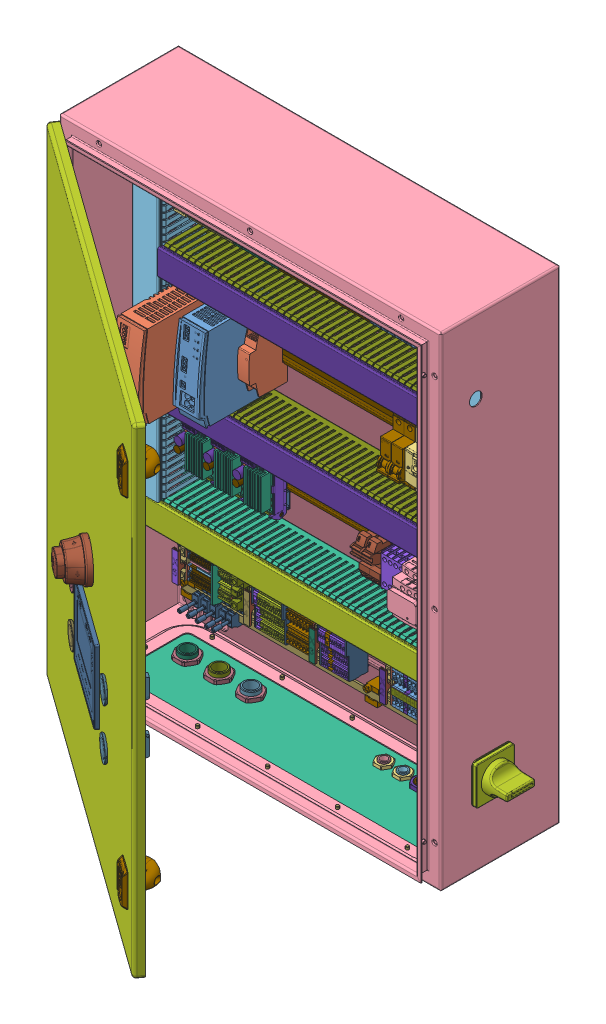
SolidWorks assembly Armoir életrique v46.step, configuration Valor predeterminado. Lengths in mm. (continued)
Components (placement in the parent): (continued)
- EM-241C_v4_1.step-1: EM-241C_v4_1.step [Valor predeterminado] at (-403.6882 -6.6708 82.3602) size (46 89.6 55.6) (continued)
  - DesignRootModel_1.step-1: DesignRootModel_1.step [Valor predeterminado] at origin size (42 72 25.9) (continued)
    - Submodel-RES0805_10K_part_simplified_0805_4.step-1: Submodel-RES0805_10K_part_simplified_0805_4.step [Valor predeterminado] at (555.4382 265.214 -26.9602) x (-1 0 0) z (0 0 1) size (2 1.25 0.6) (continued)
      - Submodel-C_UsersTino Hellbergworks3D kokeilujaEM-241Cver4_PCB3DInput_SRES 0805.xtd_76.step-1: Submodel-C_UsersTino Hellbergworks3D kokeilujaEM-241Cver4_PCB3DInput_SRES 0805.xtd_76.step [Valor predeterminado] at (-0.975 -0.625 0.025) x (1 0 0) z (0 -1 0) size (2 0.6 1.25)
        - RES 0805.step-1: RES 0805.step [Valor predeterminado] at origin size (2 0.6 1.25)
    - Submodel-RES0805_10K_part_simplified_0805_5.step-1: Submodel-RES0805_10K_part_simplified_0805_5.step [Valor predeterminado] at (555.4382 274.464 -26.9602) size (2 1.25 0.6)
      - Submodel-C_UsersTino Hellbergworks3D kokeilujaEM-241Cver4_PCB3DInput_SRES 0805.xtd_77.step-1: Submodel-C_UsersTino Hellbergworks3D kokeilujaEM-241Cver4_PCB3DInput_SRES 0805.xtd_77.step [Valor predeterminado] at (-0.975 -0.625 0.025) x (1 0 0) z (0 -1 0) size (2 0.6 1.25)
        - RES 0805.step-1: RES 0805.step [Valor predeterminado] at origin size (2 0.6 1.25)
    - Submodel-RES0805_10K_part_simplified_0805_6.step-1: Submodel-RES0805_10K_part_simplified_0805_6.step [Valor predeterminado] at (555.4382 272.714 -26.9602) size (2 1.25 0.6)
      - Submodel-C_UsersTino Hellbergworks3D kokeilujaEM-241Cver4_PCB3DInput_SRES 0805.xtd_78.step-1: Submodel-C_UsersTino Hellbergworks3D kokeilujaEM-241Cver4_PCB3DInput_SRES 0805.xtd_78.step [Valor predeterminado] at (-0.975 -0.625 0.025) x (1 0 0) z (0 -1 0) size (2 0.6 1.25)
        - RES 0805.step-1: RES 0805.step [Valor predeterminado] at origin size (2 0.6 1.25)
    - Submodel-RES0805_10K_part_simplified_0805_7.step-1: Submodel-RES0805_10K_part_simplified_0805_7.step [Valor predeterminado] at (544.6882 264.714 -26.9602) x (0 1 0) z (0 0 1) size (2 1.25 0.6)
      - Submodel-C_UsersTino Hellbergworks3D kokeilujaEM-241Cver4_PCB3DInput_SRES 0805.xtd_79.step-1: Submodel-C_UsersTino Hellbergworks3D kokeilujaEM-241Cver4_PCB3DInput_SRES 0805.xtd_79.step [Valor predeterminado] at (-0.975 -0.625 0.025) x (1 0 0) z (0 -1 0) size (2 0.6 1.25)
        - RES 0805.step-1: RES 0805.step [Valor predeterminado] at origin size (2 0.6 1.25)
    - Submodel-RES1206_10R_part_simplified_1206_1.step-1: Submodel-RES1206_10R_part_simplified_1206_1.step [Valor predeterminado] at (548.9382 260.964 -26.9602) size (3.35 1.73 0.85)
      - Submodel-C_UsersTino Hellbergworks3D kokeilujaEM-241Cver4_PCB3DInput_SRES-1206.xtd_2.step-1: Submodel-C_UsersTino Hellbergworks3D kokeilujaEM-241Cver4_PCB3DInput_SRES-1206.xtd_2.step [Valor predeterminado] x (1 0 0) z (0 -1 0) size (3.35 0.85 1.73)
        - RES-1206.step-1: RES-1206.step [Valor predeterminado] at origin size (3.35 0.85 1.73)
    - Submodel-RES0805_1K_part_simplified_0805_2.step-1: Submodel-RES0805_1K_part_simplified_0805_2.step [Valor predeterminado] at (555.4382 263.464 -26.9602) x (-1 0 0) z (0 0 1) size (2 1.25 0.6)
      - Submodel-C_UsersTino Hellbergworks3D kokeilujaEM-241Cver4_PCB3DInput_SRES 0805.xtd_80.step-1: Submodel-C_UsersTino Hellbergworks3D kokeilujaEM-241Cver4_PCB3DInput_SRES 0805.xtd_80.step [Valor predeterminado] at (-0.975 -0.625 0.025) x (1 0 0) z (0 -1 0) size (2 0.6 1.25)
        - RES 0805.step-1: RES 0805.step [Valor predeterminado] at origin size (2 0.6 1.25)
    - Submodel-RES0805_1K_part_simplified_0805_3.step-1: Submodel-RES0805_1K_part_simplified_0805_3.step [Valor predeterminado] at (548.9382 285.714 -26.9602) x (0 1 0) z (0 0 1) size (2 1.25 0.6)
      - Submodel-C_UsersTino Hellbergworks3D kokeilujaEM-241Cver4_PCB3DInput_SRES 0805.xtd_81.step-1: Submodel-C_UsersTino Hellbergworks3D kokeilujaEM-241Cver4_PCB3DInput_SRES 0805.xtd_81.step [Valor predeterminado] at (-0.975 -0.625 0.025) x (1 0 0) z (0 -1 0) size (2 0.6 1.25)
        - RES 0805.step-1: RES 0805.step [Valor predeterminado] at origin size (2 0.6 1.25)
    - Submodel-RES1206_100R_part_simplified_1206_1.step-1: Submodel-RES1206_100R_part_simplified_1206_1.step [Valor predeterminado] at (548.1882 264.714 -26.9602) x (0 1 0) z (0 0 1) size (3.35 1.73 0.85)
      - Submodel-C_UsersTino Hellbergworks3D kokeilujaEM-241Cver4_PCB3DInput_SRES-1206.xtd_3.step-1: Submodel-C_UsersTino Hellbergworks3D kokeilujaEM-241Cver4_PCB3DInput_SRES-1206.xtd_3.step [Valor predeterminado] x (1 0 0) z (0 -1 0) size (3.35 0.85 1.73)
        - RES-1206.step-1: RES-1206.step [Valor predeterminado] at origin size (3.35 0.85 1.73)
    - Submodel-RES0805_220R_part_simplified_0805_2.step-1: Submodel-RES0805_220R_part_simplified_0805_2.step [Valor predeterminado] at (555.4382 286.214 -26.9602) x (0 1 0) z (0 0 1) size (2 1.25 0.6)
      - Submodel-C_UsersTino Hellbergworks3D kokeilujaEM-241Cver4_PCB3DInput_SRES 0805.xtd_82.step-1: Submodel-C_UsersTino Hellbergworks3D kokeilujaEM-241Cver4_PCB3DInput_SRES 0805.xtd_82.step [Valor predeterminado] at (-0.975 -0.625 0.025) x (1 0 0) z (0 -1 0) size (2 0.6 1.25)
        - RES 0805.step-1: RES 0805.step [Valor predeterminado] at origin size (2 0.6 1.25)
    - Submodel-RES0805_220R_part_simplified_0805_3.step-1: Submodel-RES0805_220R_part_simplified_0805_3.step [Valor predeterminado] at (553.4382 286.214 -26.9602) x (0 1 0) z (0 0 1) size (2 1.25 0.6)
      - Submodel-C_UsersTino Hellbergworks3D kokeilujaEM-241Cver4_PCB3DInput_SRES 0805.xtd_83.step-1: Submodel-C_UsersTino Hellbergworks3D kokeilujaEM-241Cver4_PCB3DInput_SRES 0805.xtd_83.step [Valor predeterminado] at (-0.975 -0.625 0.025) x (1 0 0) z (0 -1 0) size (2 0.6 1.25)
        - RES 0805.step-1: RES 0805.step [Valor predeterminado] at origin size (2 0.6 1.25)
    - Submodel-RES0805_2K2_part_simplified_0805_7.step-1: Submodel-RES0805_2K2_part_simplified_0805_7.step [Valor predeterminado] at (516.9382 280.964 -26.9602) x (0 -1 0) z (0 0 1) size (2 1.25 0.6)
      - Submodel-C_UsersTino Hellbergworks3D kokeilujaEM-241Cver4_PCB3DInput_SRES 0805.xtd_84.step-1: Submodel-C_UsersTino Hellbergworks3D kokeilujaEM-241Cver4_PCB3DInput_SRES 0805.xtd_84.step [Valor predeterminado] at (-0.975 -0.625 0.025) x (1 0 0) z (0 -1 0) size (2 0.6 1.25)
        - RES 0805.step-1: RES 0805.step [Valor predeterminado] at origin size (2 0.6 1.25)
    - Submodel-RES0805_2K2_part_simplified_0805_8.step-1: Submodel-RES0805_2K2_part_simplified_0805_8.step [Valor predeterminado] at (542.9382 264.714 -26.9602) x (0 -1 0) z (0 0 1) size (2 1.25 0.6)
      - Submodel-C_UsersTino Hellbergworks3D kokeilujaEM-241Cver4_PCB3DInput_SRES 0805.xtd_85.step-1: Submodel-C_UsersTino Hellbergworks3D kokeilujaEM-241Cver4_PCB3DInput_SRES 0805.xtd_85.step [Valor predeterminado] at (-0.975 -0.625 0.025) x (1 0 0) z (0 -1 0) size (2 0.6 1.25)
        - RES 0805.step-1: RES 0805.step [Valor predeterminado] at origin size (2 0.6 1.25)
    - Submodel-RES0805_2K2_part_simplified_0805_9.step-1: Submodel-RES0805_2K2_part_simplified_0805_9.step [Valor predeterminado] at (519.1882 261.214 -26.9602) x (-1 0 0) z (0 0 1) size (2 1.25 0.6)
      - Submodel-C_UsersTino Hellbergworks3D kokeilujaEM-241Cver4_PCB3DInput_SRES 0805.xtd_86.step-1: Submodel-C_UsersTino Hellbergworks3D kokeilujaEM-241Cver4_PCB3DInput_SRES 0805.xtd_86.step [Valor predeterminado] at (-0.975 -0.625 0.025) x (1 0 0) z (0 -1 0) size (2 0.6 1.25)
        - RES 0805.step-1: RES 0805.step [Valor predeterminado] at origin size (2 0.6 1.25)
    - Submodel-RES0805_2K2_part_simplified_0805_10.step-1: Submodel-RES0805_2K2_part_simplified_0805_10.step [Valor predeterminado] at (524.6882 271.714 -26.9602) x (-1 0 0) z (0 0 1) size (2 1.25 0.6)
      - Submodel-C_UsersTino Hellbergworks3D kokeilujaEM-241Cver4_PCB3DInput_SRES 0805.xtd_87.step-1: Submodel-C_UsersTino Hellbergworks3D kokeilujaEM-241Cver4_PCB3DInput_SRES 0805.xtd_87.step [Valor predeterminado] at (-0.975 -0.625 0.025) x (1 0 0) z (0 -1 0) size (2 0.6 1.25)
        - RES 0805.step-1: RES 0805.step [Valor predeterminado] at origin size (2 0.6 1.25)
    - Submodel-RES0805_2K2_part_simplified_0805_11.step-1: Submodel-RES0805_2K2_part_simplified_0805_11.step [Valor predeterminado] at (550.9382 285.714 -26.9602) x (0 1 0) z (0 0 1) size (2 1.25 0.6)
      - Submodel-C_UsersTino Hellbergworks3D kokeilujaEM-241Cver4_PCB3DInput_SRES 0805.xtd_88.step-1: Submodel-C_UsersTino Hellbergworks3D kokeilujaEM-241Cver4_PCB3DInput_SRES 0805.xtd_88.step [Valor predeterminado] at (-0.975 -0.625 0.025) x (1 0 0) z (0 -1 0) size (2 0.6 1.25)
        - RES 0805.step-1: RES 0805.step [Valor predeterminado] at origin size (2 0.6 1.25)
    - Submodel-RES0805_2K2_part_simplified_0805_12.step-1: Submodel-RES0805_2K2_part_simplified_0805_12.step [Valor predeterminado] at (553.9382 283.714 -26.9602) x (-1 0 0) z (0 0 1) size (2 1.25 0.6)
      - Submodel-C_UsersTino Hellbergworks3D kokeilujaEM-241Cver4_PCB3DInput_SRES 0805.xtd_89.step-1: Submodel-C_UsersTino Hellbergworks3D kokeilujaEM-241Cver4_PCB3DInput_SRES 0805.xtd_89.step [Valor predeterminado] at (-0.975 -0.625 0.025) x (1 0 0) z (0 -1 0) size (2 0.6 1.25)
        - RES 0805.step-1: RES 0805.step [Valor predeterminado] at origin size (2 0.6 1.25)
    - Submodel-RES0805_2K2_part_simplified_0805_13.step-1: Submodel-RES0805_2K2_part_simplified_0805_13.step [Valor predeterminado] at (550.4382 258.214 -26.9602) x (0 1 0) z (0 0 1) size (2 1.25 0.6)
      - Submodel-C_UsersTino Hellbergworks3D kokeilujaEM-241Cver4_PCB3DInput_SRES 0805.xtd_90.step-1: Submodel-C_UsersTino Hellbergworks3D kokeilujaEM-241Cver4_PCB3DInput_SRES 0805.xtd_90.step [Valor predeterminado] at (-0.975 -0.625 0.025) x (1 0 0) z (0 -1 0) size (2 0.6 1.25)
        - RES 0805.step-1: RES 0805.step [Valor predeterminado] at origin size (2 0.6 1.25)
    - Submodel-PTC_1210_0.1A30V_part_simplified_1210_1.step-1: Submodel-PTC_1210_0.1A30V_part_simplified_1210_1.step [Valor predeterminado] at (527.9382 291.714 -26.9602) x (0 -1 0) z (0 0 1) size (3.2 2.5 1.5)
      - Submodel-C_UsersTino Hellbergworks3D kokeilujaEM-241Cver4_PCB3DInput_SV-1210-HD.xtd_1.step-1: Submodel-C_UsersTino Hellbergworks3D kokeilujaEM-241Cver4_PCB3DInput_SV-1210-HD.xtd_1.step [Valor predeterminado] at origin size (3.2 2.5 1.5)
        - V-1210-HD.step-1: V-1210-HD.step [Valor predeterminado] at origin size (3.2 2.5 1.5)
    - Submodel-NTC_0805_100K_part_simplified_0805_1.step-1: Submodel-NTC_0805_100K_part_simplified_0805_1.step [Valor predeterminado] at (531.6882 273.464 -26.9602) size (2 1.25 0.6)
      - Submodel-C_UsersTino Hellbergworks3D kokeilujaEM-241Cver4_PCB3DInput_SRES 0805.xtd_91.step-1: Submodel-C_UsersTino Hellbergworks3D kokeilujaEM-241Cver4_PCB3DInput_SRES 0805.xtd_91.step [Valor predeterminado] at (-0.975 -0.625 0.025) x (1 0 0) z (0 -1 0) size (2 0.6 1.25)
        - RES 0805.step-1: RES 0805.step [Valor predeterminado] at origin size (2 0.6 1.25)
    - Submodel-ATMEGA328P-AU_TQFP32_part_simplified_TQFP32_1.step-1: Submodel-ATMEGA328P-AU_TQFP32_part_simplified_TQFP32_1.step [Valor predeterminado] at (544.4382 274.714 -26.9602) x (-1 0 0) z (0 0 1) size (9.02 9.02 1.15)
      - Submodel-C_UsersTino Hellbergworks3D kokeilujaEM-241Cver4_PCB3DInput_STQFP32.xtd_1.step-1: Submodel-C_UsersTino Hellbergworks3D kokeilujaEM-241Cver4_PCB3DInput_STQFP32.xtd_1.step [Valor predeterminado] at (0 0 0.1493) x (1 0 0) z (0 -1 0) size (9.02 1.15 9.02)
        - TQFP32.step-1: TQFP32.step [Valor predeterminado] at origin size (9.02 1.15 9.02)
    - Submodel-HS_SK177-50SA_28.0X50.0_7CW_part_simplified_HS-SK177-50SA_1.step-1: Submodel-HS_SK177-50SA_28.0X50.0_7CW_part_simplified_HS-SK177-50SA_1.step [Valor predeterminado] at (557.6882 312.214 -26.9602) x (-1 0 0) z (0 0 1) size (27.94 50 15.24)
      - Submodel-C_UsersTino Hellbergworks3D kokeilujaEM-241Cver4_PCB3DInput_S-SK177-50.xtd_1.step-1: Submodel-C_UsersTino Hellbergworks3D kokeilujaEM-241Cver4_PCB3DInput_S-SK177-50.xtd_1.step [Valor predeterminado] at (0.03 -0.5 2.4) size (27.94 50 15.24)
        - PV-SK177-50.step-1: PV-SK177-50.step [Valor predeterminado] at origin size (27.94 50 15.24)
    - Submodel-BZV55-C6V2_ZENER-6.2V-0.5W_part_simplified_SOD80_1.step-1: Submodel-BZV55-C6V2_ZENER-6.2V-0.5W_part_simplified_SOD80_1.step [Valor predeterminado] at (528.6882 275.214 -26.9602) x (0 1 0) z (0 0 1) size (3.7 1.6 1.6)
      - Submodel-C_UsersTino Hellbergworks3D kokeilujaEM-241Cver4_PCB3DInput_SOD80.xtd_3.step-1: Submodel-C_UsersTino Hellbergworks3D kokeilujaEM-241Cver4_PCB3DInput_SOD80.xtd_3.step [Valor predeterminado] at (0.03 0 0) size (3.7 1.6 1.6)
        - SOD80.step-1: SOD80.step [Valor predeterminado] at origin size (3.7 1.6 1.6)
    - Submodel-US1J_1A600V_SMA_part_simplified_SMA_1.step-1: Submodel-US1J_1A600V_SMA_part_simplified_SMA_1.step [Valor predeterminado] at (536.4382 283.964 -26.9602) x (0 1 0) z (0 0 1) size (5.2 2.6 2.45)
      - Submodel-C_UsersTino Hellbergworks3D kokeilujaEM-241Cver4_PCB3DInput_SDO-214AC SMA.xtd_1.step-1: Submodel-C_UsersTino Hellbergworks3D kokeilujaEM-241Cver4_PCB3DInput_SDO-214AC SMA.xtd_1.step [Valor predeterminado] at (0 0 1.4) x (0 1 0) z (0 0 1) size (2.6 5.2 2.45)
        - DO-214AC SMA.step-1: DO-214AC SMA.step [Valor predeterminado] at origin size (2.6 5.2 2.45)
    - Submodel-BAS70-04W_0.07A70V-DUAL-SCHOTT_part_simplified_SOT323_2.step-1: Submodel-BAS70-04W_0.07A70V-DUAL-SCHOTT_part_simplified_SOT323_2.step [Valor predeterminado] at (540.6882 298.714 -26.9602) x (0 -1 0) z (0 0 1) size (2.1 2.3 1)
      - Submodel-C_UsersTino Hellbergworks3D kokeilujaEM-241Cver4_PCB3DInput_SOT-323.xtd_2.step-1: Submodel-C_UsersTino Hellbergworks3D kokeilujaEM-241Cver4_PCB3DInput_SOT-323.xtd_2.step [Valor predeterminado] at (0 0.0625 0) size (2.1 2.3 1)
        - SOT-323.step-1: SOT-323.step [Valor predeterminado] at origin size (2.1 2.3 1)
    - Submodel-BAS70-04W_0.07A70V-DUAL-SCHOTT_part_simplified_SOT323_3.step-1: Submodel-BAS70-04W_0.07A70V-DUAL-SCHOTT_part_simplified_SOT323_3.step [Valor predeterminado] at (540.6882 291.214 -26.9602) x (0 -1 0) z (0 0 1) size (2.1 2.3 1)
      - Submodel-C_UsersTino Hellbergworks3D kokeilujaEM-241Cver4_PCB3DInput_SOT-323.xtd_3.step-1: Submodel-C_UsersTino Hellbergworks3D kokeilujaEM-241Cver4_PCB3DInput_SOT-323.xtd_3.step [Valor predeterminado] at (0 0.0625 0) size (2.1 2.3 1)
        - SOT-323.step-1: SOT-323.step [Valor predeterminado] at origin size (2.1 2.3 1)
    - Submodel-LS4148_0.2A100V_SOD80_part_simplified_SOD80_2.step-1: Submodel-LS4148_0.2A100V_SOD80_part_simplified_SOD80_2.step [Valor predeterminado] at (549.6882 304.714 -26.9602) size (3.7 1.6 1.6)
      - Submodel-C_UsersTino Hellbergworks3D kokeilujaEM-241Cver4_PCB3DInput_SOD80.xtd_4.step-1: Submodel-C_UsersTino Hellbergworks3D kokeilujaEM-241Cver4_PCB3DInput_SOD80.xtd_4.step [Valor predeterminado] at (0.03 0 0) size (3.7 1.6 1.6)
        - SOD80.step-1: SOD80.step [Valor predeterminado] at origin size (3.7 1.6 1.6)
    - Submodel-LS4148_0.2A100V_SOD80_part_simplified_SOD80_3.step-1: Submodel-LS4148_0.2A100V_SOD80_part_simplified_SOD80_3.step [Valor predeterminado] at (553.1882 281.714 -26.9602) size (3.7 1.6 1.6)
      - Submodel-C_UsersTino Hellbergworks3D kokeilujaEM-241Cver4_PCB3DInput_SOD80.xtd_5.step-1: Submodel-C_UsersTino Hellbergworks3D kokeilujaEM-241Cver4_PCB3DInput_SOD80.xtd_5.step [Valor predeterminado] at (0.03 0 0) size (3.7 1.6 1.6)
        - SOD80.step-1: SOD80.step [Valor predeterminado] at origin size (3.7 1.6 1.6)
    - Submodel-TOPLED_RED_645NM180MCD_PLCC2_part_simplified_PLCC2_1.step-1: Submodel-TOPLED_RED_645NM180MCD_PLCC2_part_simplified_PLCC2_1.step [Valor predeterminado] at (553.6882 260.964 -26.9602) x (-1 0 0) z (0 0 1) size (3.5 2.8 1.9)
      - Submodel-C_UsersTino Hellbergworks3D kokeilujaEM-241Cver4_PCB3DInput_SMD LED PLCC-2.xtd_1.step-1: Submodel-C_UsersTino Hellbergworks3D kokeilujaEM-241Cver4_PCB3DInput_SMD LED PLCC-2.xtd_1.step [Valor predeterminado] x (0 1 0) z (0 0 -1) size (2.8 3.5 1.9)
        - SMD LED PLCC-2.step-1: SMD LED PLCC-2.step [Valor predeterminado] at origin size (2.8 3.5 1.9)
    - Submodel-CAP1206_10UF_10V_part_simplified_1206_1.step-1: Submodel-CAP1206_10UF_10V_part_simplified_1206_1.step [Valor predeterminado] at (552.1882 276.464 -26.9602) size (3.4 1.8 0.88)
      - Submodel-C_UsersTino Hellbergworks3D kokeilujaEM-241Cver4_PCB3DInput_SCAP 1206.xtd_1.step-1: Submodel-C_UsersTino Hellbergworks3D kokeilujaEM-241Cver4_PCB3DInput_SCAP 1206.xtd_1.step [Valor predeterminado] at (97.4085 -43.3809 11.5241) x (1 0 0) z (0 1 0) size (3.4 0.88 1.8)
        - CAP 1206.step-1: CAP 1206.step [Valor predeterminado] at origin size (3.4 0.88 1.8)
    - Submodel-CAP0603_100NF_part_simplified_0603_4.step-1: Submodel-CAP0603_100NF_part_simplified_0603_4.step [Valor predeterminado] at (546.4382 264.464 -26.9602) x (0 1 0) z (0 0 1) size (1.75 0.95 0.87)
      - Submodel-C_UsersTino Hellbergworks3D kokeilujaEM-241Cver4_PCB3DInput_SCAP 0603.xtd_16.step-1: Submodel-C_UsersTino Hellbergworks3D kokeilujaEM-241Cver4_PCB3DInput_SCAP 0603.xtd_16.step [Valor predeterminado] at (96.5835 -43.8059 11.5141) x (1 0 0) z (0 1 0) size (1.75 0.87 0.95)
        - CAP 0603.step-1: CAP 0603.step [Valor predeterminado] at origin size (1.75 0.87 0.95)
    - Submodel-CAP0603_100NF_part_simplified_0603_5.step-1: Submodel-CAP0603_100NF_part_simplified_0603_5.step [Valor predeterminado] at (552.9382 264.464 -26.9602) x (0 -1 0) z (0 0 1) size (1.75 0.95 0.87)
      - Submodel-C_UsersTino Hellbergworks3D kokeilujaEM-241Cver4_PCB3DInput_SCAP 0603.xtd_17.step-1: Submodel-C_UsersTino Hellbergworks3D kokeilujaEM-241Cver4_PCB3DInput_SCAP 0603.xtd_17.step [Valor predeterminado] at (96.5835 -43.8059 11.5141) x (1 0 0) z (0 1 0) size (1.75 0.87 0.95)
        - CAP 0603.step-1: CAP 0603.step [Valor predeterminado] at origin size (1.75 0.87 0.95)
    - Submodel-CAP0603_100NF_part_simplified_0603_6.step-1: Submodel-CAP0603_100NF_part_simplified_0603_6.step [Valor predeterminado] at (551.4382 267.964 -26.9602) x (0 -1 0) z (0 0 1) size (1.75 0.95 0.87)
      - Submodel-C_UsersTino Hellbergworks3D kokeilujaEM-241Cver4_PCB3DInput_SCAP 0603.xtd_18.step-1: Submodel-C_UsersTino Hellbergworks3D kokeilujaEM-241Cver4_PCB3DInput_SCAP 0603.xtd_18.step [Valor predeterminado] at (96.5835 -43.8059 11.5141) x (1 0 0) z (0 1 0) size (1.75 0.87 0.95)
        - CAP 0603.step-1: CAP 0603.step [Valor predeterminado] at origin size (1.75 0.87 0.95)
    - Submodel-CAP0603_100NF_part_simplified_0603_7.step-1: Submodel-CAP0603_100NF_part_simplified_0603_7.step [Valor predeterminado] at (539.4382 278.464 -26.9602) size (1.75 0.95 0.87)
      - Submodel-C_UsersTino Hellbergworks3D kokeilujaEM-241Cver4_PCB3DInput_SCAP 0603.xtd_19.step-1: Submodel-C_UsersTino Hellbergworks3D kokeilujaEM-241Cver4_PCB3DInput_SCAP 0603.xtd_19.step [Valor predeterminado] at (96.5835 -43.8059 11.5141) x (1 0 0) z (0 1 0) size (1.75 0.87 0.95)
        - CAP 0603.step-1: CAP 0603.step [Valor predeterminado] at origin size (1.75 0.87 0.95)
    - Submodel-CAP0603_1NF_part_simplified_0603_8.step-1: Submodel-CAP0603_1NF_part_simplified_0603_8.step [Valor predeterminado] at (543.1882 289.464 -26.9602) x (0 1 0) z (0 0 1) size (1.75 0.95 0.87)
      - Submodel-C_UsersTino Hellbergworks3D kokeilujaEM-241Cver4_PCB3DInput_SCAP 0603.xtd_20.step-1: Submodel-C_UsersTino Hellbergworks3D kokeilujaEM-241Cver4_PCB3DInput_SCAP 0603.xtd_20.step [Valor predeterminado] at (96.5835 -43.8059 11.5141) x (1 0 0) z (0 1 0) size (1.75 0.87 0.95)
        - CAP 0603.step-1: CAP 0603.step [Valor predeterminado] at origin size (1.75 0.87 0.95)
    - Submodel-CAP0603_1NF_part_simplified_0603_9.step-1: Submodel-CAP0603_1NF_part_simplified_0603_9.step [Valor predeterminado] at (543.9382 281.964 -26.9602) x (0 1 0) z (0 0 1) size (1.75 0.95 0.87)
      - Submodel-C_UsersTino Hellbergworks3D kokeilujaEM-241Cver4_PCB3DInput_SCAP 0603.xtd_21.step-1: Submodel-C_UsersTino Hellbergworks3D kokeilujaEM-241Cver4_PCB3DInput_SCAP 0603.xtd_21.step [Valor predeterminado] at (96.5835 -43.8059 11.5141) x (1 0 0) z (0 1 0) size (1.75 0.87 0.95)
        - CAP 0603.step-1: CAP 0603.step [Valor predeterminado] at origin size (1.75 0.87 0.95)
    - Submodel-CAP0603_1NF_part_simplified_0603_10.step-1: Submodel-CAP0603_1NF_part_simplified_0603_10.step [Valor predeterminado] at (536.6882 277.714 -26.9602) x (0 1 0) z (0 0 1) size (1.75 0.95 0.87)
      - Submodel-C_UsersTino Hellbergworks3D kokeilujaEM-241Cver4_PCB3DInput_SCAP 0603.xtd_22.step-1: Submodel-C_UsersTino Hellbergworks3D kokeilujaEM-241Cver4_PCB3DInput_SCAP 0603.xtd_22.step [Valor predeterminado] at (96.5835 -43.8059 11.5141) x (1 0 0) z (0 1 0) size (1.75 0.87 0.95)
        - CAP 0603.step-1: CAP 0603.step [Valor predeterminado] at origin size (1.75 0.87 0.95)
    - Submodel-CAP0603_1NF_part_simplified_0603_11.step-1: Submodel-CAP0603_1NF_part_simplified_0603_11.step [Valor predeterminado] at (536.6882 274.214 -26.9602) x (0 1 0) z (0 0 1) size (1.75 0.95 0.87)
      - Submodel-C_UsersTino Hellbergworks3D kokeilujaEM-241Cver4_PCB3DInput_SCAP 0603.xtd_23.step-1: Submodel-C_UsersTino Hellbergworks3D kokeilujaEM-241Cver4_PCB3DInput_SCAP 0603.xtd_23.step [Valor predeterminado] at (96.5835 -43.8059 11.5141) x (1 0 0) z (0 1 0) size (1.75 0.87 0.95)
        - CAP 0603.step-1: CAP 0603.step [Valor predeterminado] at origin size (1.75 0.87 0.95)
    - Submodel-CAP0603_1NF_part_simplified_0603_12.step-1: Submodel-CAP0603_1NF_part_simplified_0603_12.step [Valor predeterminado] at (534.6882 274.214 -26.9602) x (0 1 0) z (0 0 1) size (1.75 0.95 0.87)
      - Submodel-C_UsersTino Hellbergworks3D kokeilujaEM-241Cver4_PCB3DInput_SCAP 0603.xtd_24.step-1: Submodel-C_UsersTino Hellbergworks3D kokeilujaEM-241Cver4_PCB3DInput_SCAP 0603.xtd_24.step [Valor predeterminado] at (96.5835 -43.8059 11.5141) x (1 0 0) z (0 1 0) size (1.75 0.87 0.95)
        - CAP 0603.step-1: CAP 0603.step [Valor predeterminado] at origin size (1.75 0.87 0.95)
    - Submodel-CAP0603_1NF_part_simplified_0603_13.step-1: Submodel-CAP0603_1NF_part_simplified_0603_13.step [Valor predeterminado] at (534.6882 277.714 -26.9602) x (0 -1 0) z (0 0 1) size (1.75 0.95 0.87)
      - Submodel-C_UsersTino Hellbergworks3D kokeilujaEM-241Cver4_PCB3DInput_SCAP 0603.xtd_25.step-1: Submodel-C_UsersTino Hellbergworks3D kokeilujaEM-241Cver4_PCB3DInput_SCAP 0603.xtd_25.step [Valor predeterminado] at (96.5835 -43.8059 11.5141) x (1 0 0) z (0 1 0) size (1.75 0.87 0.95)
        - CAP 0603.step-1: CAP 0603.step [Valor predeterminado] at origin size (1.75 0.87 0.95)
    - Submodel-CAP0603_1NF_part_simplified_0603_14.step-1: Submodel-CAP0603_1NF_part_simplified_0603_14.step [Valor predeterminado] at (545.1882 281.964 -26.9602) x (0 1 0) z (0 0 1) size (1.75 0.95 0.87)
      - Submodel-C_UsersTino Hellbergworks3D kokeilujaEM-241Cver4_PCB3DInput_SCAP 0603.xtd_26.step-1: Submodel-C_UsersTino Hellbergworks3D kokeilujaEM-241Cver4_PCB3DInput_SCAP 0603.xtd_26.step [Valor predeterminado] at (96.5835 -43.8059 11.5141) x (1 0 0) z (0 1 0) size (1.75 0.87 0.95)
        - CAP 0603.step-1: CAP 0603.step [Valor predeterminado] at origin size (1.75 0.87 0.95)
    - Submodel-CAP0603_1NF_part_simplified_0603_15.step-1: Submodel-CAP0603_1NF_part_simplified_0603_15.step [Valor predeterminado] at (543.1882 296.964 -26.9602) x (0 1 0) z (0 0 1) size (1.75 0.95 0.87)
      - Submodel-C_UsersTino Hellbergworks3D kokeilujaEM-241Cver4_PCB3DInput_SCAP 0603.xtd_27.step-1: Submodel-C_UsersTino Hellbergworks3D kokeilujaEM-241Cver4_PCB3DInput_SCAP 0603.xtd_27.step [Valor predeterminado] at (96.5835 -43.8059 11.5141) x (1 0 0) z (0 1 0) size (1.75 0.87 0.95)
        - CAP 0603.step-1: CAP 0603.step [Valor predeterminado] at origin size (1.75 0.87 0.95)
    - Submodel-CAP0603_2N2_part_simplified_0603_4.step-1: Submodel-CAP0603_2N2_part_simplified_0603_4.step [Valor predeterminado] at (543.1882 292.464 -26.9602) x (0 1 0) z (0 0 1) size (1.75 0.95 0.87)
      - Submodel-C_UsersTino Hellbergworks3D kokeilujaEM-241Cver4_PCB3DInput_SCAP 0603.xtd_28.step-1: Submodel-C_UsersTino Hellbergworks3D kokeilujaEM-241Cver4_PCB3DInput_SCAP 0603.xtd_28.step [Valor predeterminado] at (96.5835 -43.8059 11.5141) x (1 0 0) z (0 1 0) size (1.75 0.87 0.95)
        - CAP 0603.step-1: CAP 0603.step [Valor predeterminado] at origin size (1.75 0.87 0.95)
    - Submodel-CAP0603_2N2_part_simplified_0603_5.step-1: Submodel-CAP0603_2N2_part_simplified_0603_5.step [Valor predeterminado] at (554.9382 297.964 -26.9602) x (-1 0 0) z (0 0 1) size (1.75 0.95 0.87)
      - Submodel-C_UsersTino Hellbergworks3D kokeilujaEM-241Cver4_PCB3DInput_SCAP 0603.xtd_29.step-1: Submodel-C_UsersTino Hellbergworks3D kokeilujaEM-241Cver4_PCB3DInput_SCAP 0603.xtd_29.step [Valor predeterminado] at (96.5835 -43.8059 11.5141) x (1 0 0) z (0 1 0) size (1.75 0.87 0.95)
        - CAP 0603.step-1: CAP 0603.step [Valor predeterminado] at origin size (1.75 0.87 0.95)
    - Submodel-CAP0603_2N2_part_simplified_0603_6.step-1: Submodel-CAP0603_2N2_part_simplified_0603_6.step [Valor predeterminado] at (543.1882 299.964 -26.9602) x (0 1 0) z (0 0 1) size (1.75 0.95 0.87)
      - Submodel-C_UsersTino Hellbergworks3D kokeilujaEM-241Cver4_PCB3DInput_SCAP 0603.xtd_30.step-1: Submodel-C_UsersTino Hellbergworks3D kokeilujaEM-241Cver4_PCB3DInput_SCAP 0603.xtd_30.step [Valor predeterminado] at (96.5835 -43.8059 11.5141) x (1 0 0) z (0 1 0) size (1.75 0.87 0.95)
        - CAP 0603.step-1: CAP 0603.step [Valor predeterminado] at origin size (1.75 0.87 0.95)
    - Submodel-CAP0603_2N2_part_simplified_0603_7.step-1: Submodel-CAP0603_2N2_part_simplified_0603_7.step [Valor predeterminado] at (554.6882 290.464 -26.9602) x (-1 0 0) z (0 0 1) size (1.75 0.95 0.87)
      - Submodel-C_UsersTino Hellbergworks3D kokeilujaEM-241Cver4_PCB3DInput_SCAP 0603.xtd_31.step-1: Submodel-C_UsersTino Hellbergworks3D kokeilujaEM-241Cver4_PCB3DInput_SCAP 0603.xtd_31.step [Valor predeterminado] at (96.5835 -43.8059 11.5141) x (1 0 0) z (0 1 0) size (1.75 0.87 0.95)
        - CAP 0603.step-1: CAP 0603.step [Valor predeterminado] at origin size (1.75 0.87 0.95)
    - Submodel-7-215079-6_V_CON_MICROMATCH6_part_DIL6-V-2.54-MMATCH_1.step-1: Submodel-7-215079-6_V_CON_MICROMATCH6_part_DIL6-V-2.54-MMATCH_1.step [Valor predeterminado] at (519.6882 267.464 -26.9602) x (0 1 0) z (0 0 1) size (9.56 5 7.15)
      - Submodel-C_UsersTino Hellbergworks3D kokeilujaEM-241Cver4_PCB3DImportedPartModelsc-7-215079-6-t-3d.step_1.step-1: Submodel-C_UsersTino Hellbergworks3D kokeilujaEM-241Cver4_PCB3DImportedPartModelsc-7-215079-6-t-3d.step_1.step [Valor predeterminado] at (0.0125 0 4.05) size (9.56 5 7.15)
        - c-7-215079-6-t-3d.step.step-1: c-7-215079-6-t-3d.step.step [Valor predeterminado] at origin size (9.56 5 7.15)
    - Submodel-PT1.5_slash_3-3.5-H_part_CON-H3-7.6_slash_9.2_slash_3.5_2.step-1: Submodel-PT1.5_slash_3-3.5-H_part_CON-H3-7.6_slash_9.2_slash_3.5_2.step [Valor predeterminado] at (527.414 259.464 -26.9602) size (11.2 7.55 13.65)
      - Submodel-C_UsersTino Hellbergworks3D kokeilujaEM-241Cver4_PCB3DImportedPartModelspxc_1984620_01_PT-1-5-3-3-5-H_3D.stp_2.step-1: Submodel-C_UsersTino Hellbergworks3D kokeilujaEM-241Cver4_PCB3DImportedPartModelspxc_1984620_01_PT-1-5-3-3-5-H_3D.stp_2.step [Valor predeterminado] at (-5.32 -3.925 0) size (11.2 7.55 13.65)
        - pxc_1984620_01_PT-1-5-3-3-5-H_3D.stp.step-1: pxc_1984620_01_PT-1-5-3-3-5-H_3D.stp.step [Valor predeterminado] at origin size (11.2 7.55 13.65)
    - Submodel-PT1.5_slash_2-3.5-H_part_CON-H2-7.6_slash_9.2_slash_3.5_2.step-1: Submodel-PT1.5_slash_2-3.5-H_part_CON-H2-7.6_slash_9.2_slash_3.5_2.step [Valor predeterminado] at (536.1644 259.464 -26.9602) size (7.7 7.55 13.65)
      - Submodel-C_UsersTino Hellbergworks3D kokeilujaEM-241Cver4_PCB3DImportedPartModelspxc_1984617_01_PT-1-5-2-3-5-H_3D.stp_2.step-1: Submodel-C_UsersTino Hellbergworks3D kokeilujaEM-241Cver4_PCB3DImportedPartModelspxc_1984617_01_PT-1-5-2-3-5-H_3D.stp_2.step [Valor predeterminado] at (-3.52 -3.925 0) size (7.7 7.55 13.65)
        - pxc_1984617_01_PT-1-5-2-3-5-H_3D.stp.step-1: pxc_1984617_01_PT-1-5-2-3-5-H_3D.stp.step [Valor predeterminado] at origin size (7.7 7.55 13.65)
    - Submodel-PT1.5_slash_2-3.5-H_part_CON-H2-7.6_slash_9.2_slash_3.5_3.step-1: Submodel-PT1.5_slash_2-3.5-H_part_CON-H2-7.6_slash_9.2_slash_3.5_3.step [Valor predeterminado] at (543.1686 259.464 -26.9602) size (7.7 7.55 13.65)
      - Submodel-C_UsersTino Hellbergworks3D kokeilujaEM-241Cver4_PCB3DImportedPartModelspxc_1984617_01_PT-1-5-2-3-5-H_3D.stp_3.step-1: Submodel-C_UsersTino Hellbergworks3D kokeilujaEM-241Cver4_PCB3DImportedPartModelspxc_1984617_01_PT-1-5-2-3-5-H_3D.stp_3.step [Valor predeterminado] at (-3.52 -3.925 0) size (7.7 7.55 13.65)
        - pxc_1984617_01_PT-1-5-2-3-5-H_3D.stp.step-1: pxc_1984617_01_PT-1-5-2-3-5-H_3D.stp.step [Valor predeterminado] at origin size (7.7 7.55 13.65)
    - Submodel-PT1.5_slash_3-3.5-H_part_CON-H3-7.6_slash_9.2_slash_3.5_3.step-1: Submodel-PT1.5_slash_3-3.5-H_part_CON-H3-7.6_slash_9.2_slash_3.5_3.step [Valor predeterminado] at (546.9382 317.414 -26.9602) x (-1 0 0) z (0 0 1) size (11.2 7.55 13.65)
      - Submodel-C_UsersTino Hellbergworks3D kokeilujaEM-241Cver4_PCB3DImportedPartModelspxc_1984620_01_PT-1-5-3-3-5-H_3D.stp_3.step-1: Submodel-C_UsersTino Hellbergworks3D kokeilujaEM-241Cver4_PCB3DImportedPartModelspxc_1984620_01_PT-1-5-3-3-5-H_3D.stp_3.step [Valor predeterminado] at (-5.32 -3.925 0) size (11.2 7.55 13.65)
        - pxc_1984620_01_PT-1-5-3-3-5-H_3D.stp.step-1: pxc_1984620_01_PT-1-5-3-3-5-H_3D.stp.step [Valor predeterminado] at origin size (11.2 7.55 13.65)
    - Submodel-22-27-2071_V_MOLEX7-HEADER_2818368710_part_SIL7-V-2.54-MOLEX_NOSILK_1.step-1: Submodel-22-27-2071_V_MOLEX7-HEADER_2818368710_part_SIL7-V-2.54-MOLEX_NOSILK_1.step [Valor predeterminado] at (536.1882 256.614 -26.9602) size (17.78 5.8 0.01)
      - Submodel-noModelForPart_22-27-2071_V_MOLEX7-HEADER_2818368710_1.step-1: Submodel-noModelForPart_22-27-2071_V_MOLEX7-HEADER_2818368710_1.step [Valor predeterminado] at origin size (17.78 5.8 0.01)
        - placementOutline.step-1: placementOutline.step [Valor predeterminado] at origin size (5.08 0.5 0.01)
        - placementOutline (1).step-1: placementOutline (1).step [Valor predeterminado] at origin size (5.08 1 0.01)
        - placementOutline (2).step-1: placementOutline (2).step [Valor predeterminado] at origin size (0.6 0.6 0.01)
        - placementOutline (3).step-1: placementOutline (3).step [Valor predeterminado] at origin size (0.3 0.3 0.01)
        - placementOutline (4).step-1: placementOutline (4).step [Valor predeterminado] at origin size (0.6 0.6 0.01)
        - placementOutline (5).step-1: placementOutline (5).step [Valor predeterminado] at origin size (0.3 0.3 0.01)
        - placementOutline (6).step-1: placementOutline (6).step [Valor predeterminado] at origin size (0.3 0.3 0.01)
        - placementOutline (7).step-1: placementOutline (7).step [Valor predeterminado] at origin size (0.6 0.6 0.01)
        - placementOutline (8).step-1: placementOutline (8).step [Valor predeterminado] at origin size (0.6 0.6 0.01)
        - placementOutline (9).step-1: placementOutline (9).step [Valor predeterminado] at origin size (0.3 0.3 0.01)
        - placementOutline (10).step-1: placementOutline (10).step [Valor predeterminado] at origin size (17.78 5.8 0.01)
        - placementOutline (11).step-1: placementOutline (11).step [Valor predeterminado] at origin size (5.08 0.5 0.01)
        - placementOutline (12).step-1: placementOutline (12).step [Valor predeterminado] at origin size (5.08 1 0.01)
        - placementOutline (13).step-1: placementOutline (13).step [Valor predeterminado] at origin size (0.6 0.6 0.01)
        - placementOutline (14).step-1: placementOutline (14).step [Valor predeterminado] at origin size (0.3 0.3 0.01)
        - placementOutline (15).step-1: placementOutline (15).step [Valor predeterminado] at origin size (0.6 0.6 0.01)
        - placementOutline (16).step-1: placementOutline (16).step [Valor predeterminado] at origin size (0.3 0.3 0.01)
        - placementOutline (17).step-1: placementOutline (17).step [Valor predeterminado] at origin size (0.3 0.3 0.01)
        - placementOutline (18).step-1: placementOutline (18).step [Valor predeterminado] at origin size (0.6 0.6 0.01)
    - Submodel-PT2.5_slash_2-5.0-H_part_CON-H2-9_slash_13.5_slash_5.0_2.step-1: Submodel-PT2.5_slash_2-5.0-H_part_CON-H2-9_slash_13.5_slash_5.0_2.step [Valor predeterminado] at (525.9515 318.214 -26.9602) x (-1 0 0) z (0 0 1) size (10 9 17.6)
      - Submodel-C_UsersTino Hellbergworks3D kokeilujaEM-241Cver4_PCB3DImportedPartModelspxc_1935776_00_PT-2-5-2-5-0-H_3D.stp_2.step-1: Submodel-C_UsersTino Hellbergworks3D kokeilujaEM-241Cver4_PCB3DImportedPartModelspxc_1935776_00_PT-2-5-2-5-0-H_3D.stp_2.step [Valor predeterminado] at (13.9475 50.6993 -15.5526) x (0 -1 0) z (-1 0 0) size (9 17.6 10)
        - pxc_1935776_00_PT-2-5-2-5-0-H_3D.stp.step-1: pxc_1935776_00_PT-2-5-2-5-0-H_3D.stp.step [Valor predeterminado] at origin size (9 17.6 10)
    - Submodel-PT2.5_slash_2-5.0-H_part_CON-H2-9_slash_13.5_slash_5.0_3.step-1: Submodel-PT2.5_slash_2-5.0-H_part_CON-H2-9_slash_13.5_slash_5.0_3.step [Valor predeterminado] at (535.9318 318.214 -26.9602) x (-1 0 0) z (0 0 1) size (10 9 17.6)
      - Submodel-C_UsersTino Hellbergworks3D kokeilujaEM-241Cver4_PCB3DImportedPartModelspxc_1935776_00_PT-2-5-2-5-0-H_3D.stp_3.step-1: Submodel-C_UsersTino Hellbergworks3D kokeilujaEM-241Cver4_PCB3DImportedPartModelspxc_1935776_00_PT-2-5-2-5-0-H_3D.stp_3.step [Valor predeterminado] at (13.9475 50.6993 -15.5526) x (0 -1 0) z (-1 0 0) size (9 17.6 10)
        - pxc_1935776_00_PT-2-5-2-5-0-H_3D.stp.step-1: pxc_1935776_00_PT-2-5-2-5-0-H_3D.stp.step [Valor predeterminado] at origin size (9 17.6 10)
    - Submodel-22-27-2031_V_MOLEX3-HEADER_3592429379_part_SIL3-V-2.54-MOLEX_NOSILK_1.step-1: Submodel-22-27-2031_V_MOLEX3-HEADER_3592429379_part_SIL3-V-2.54-MOLEX_NOSILK_1.step [Valor predeterminado] at (546.9382 320.214 -26.9602) x (-1 0 0) z (0 0 1) size (7.6 5.8 0.01)
      - Submodel-noModelForPart_22-27-2031_V_MOLEX3-HEADER_3592429379_1.step-1: Submodel-noModelForPart_22-27-2031_V_MOLEX3-HEADER_3592429379_1.step [Valor predeterminado] at origin size (7.6 5.8 0.01)
        - placementOutline (19).step-1: placementOutline (19).step [Valor predeterminado] at origin size (7.6 5.8 0.01)
        - placementOutline (20).step-1: placementOutline (20).step [Valor predeterminado] at origin size (5.1 0.5 0.01)
        - placementOutline (21).step-1: placementOutline (21).step [Valor predeterminado] at origin size (5.1 1 0.01)
        - placementOutline (22).step-1: placementOutline (22).step [Valor predeterminado] at origin size (0.6 0.6 0.01)
        - placementOutline (23).step-1: placementOutline (23).step [Valor predeterminado] at origin size (0.3 0.3 0.01)
        - placementOutline (24).step-1: placementOutline (24).step [Valor predeterminado] at origin size (0.6 0.6 0.01)
        - placementOutline (25).step-1: placementOutline (25).step [Valor predeterminado] at origin size (0.3 0.3 0.01)
        - placementOutline (26).step-1: placementOutline (26).step [Valor predeterminado] at origin size (0.3 0.3 0.01)
        - placementOutline (27).step-1: placementOutline (27).step [Valor predeterminado] at origin size (0.6 0.6 0.01)
    - Submodel-SIL-SOCKET_2_RIBBON-2.54_part_SIL2-V-2.54_1.step-1: Submodel-SIL-SOCKET_2_RIBBON-2.54_part_SIL2-V-2.54_1.step [Valor predeterminado] at (548.4282 257.404 -26.9602) x (0 1 0) z (0 0 1) size (5.08 2.54 7.37)
      - Submodel-C_UsersTino Hellbergworks3D kokeilujaEM-241Cver4_PCB3DImportedPartModelssil socket 2-way.STEP_1.step-1: Submodel-C_UsersTino Hellbergworks3D kokeilujaEM-241Cver4_PCB3DImportedPartModelssil socket 2-way.STEP_1.step [Valor predeterminado] at (-2.615 0.9644 4.266) x (0 -1 0) z (-1 0 0) size (2.54 7.37 5.08)
        - sil socket 2-way.STEP.step-1: sil socket 2-way.STEP.step [Valor predeterminado] at origin size (2.54 7.37 5.08)
    - Submodel-VDR_RAD_30VAC38VDC2J_1196060662_part_VDR-RAD-7.6_slash_2.6_slash_5.1_1.step-1: Submodel-VDR_RAD_30VAC38VDC2J_1196060662_part_VDR-RAD-7.6_slash_2.6_slash_5.1_1.step [Valor predeterminado] at (518.6882 310.214 -26.9602) x (0 -1 0) z (0 0 1) size (7.28 3.6 7)
      - Submodel-noModelForPart_VDR_RAD_30VAC38VDC2J_1196060662_1.step-1: Submodel-noModelForPart_VDR_RAD_30VAC38VDC2J_1196060662_1.step [Valor predeterminado] at origin size (7.28 3.6 7)
        - placementOutline (28).step-1: placementOutline (28).step [Valor predeterminado] at origin size (7.28 3.6 7)
    - Submodel-NHDS-4_SMD-6.3_slash_6.7_slash_1.5_DIP4_part_SW-DIP4-6.3_slash_6.7_slash_1.5_1.step-1: Submodel-NHDS-4_SMD-6.3_slash_6.7_slash_1.5_DIP4_part_SW-DIP4-6.3_slash_6.7_slash_1.5_1.step [Valor predeterminado] at (520.4382 275.714 -26.9602) x (0 -1 0) z (0 0 1) size (6.31 6.7 1.59)
      - Submodel-C_UsersTino Hellbergworks3D kokeilujaEM-241Cver4_PCB3DImportedPartModelsMCDHN-04.step_1.step-1: Submodel-C_UsersTino Hellbergworks3D kokeilujaEM-241Cver4_PCB3DImportedPartModelsMCDHN-04.step_1.step [Valor predeterminado] at (0.04 0.05 0.075) size (6.31 6.7 1.59)
        - MCDHN-04.step.step-1: MCDHN-04.step.step [Valor predeterminado] at origin size (6.31 6.7 1.59)
    - Submodel-RES1206_47R_part_1206_1.step-1: Submodel-RES1206_47R_part_1206_1.step [Valor predeterminado] at (554.4382 315.964 -26.9602) x (0 1 0) z (0 0 1) size (3.35 1.73 0.85)
      - Submodel-C_UsersTino Hellbergworks3D kokeilujaEM-241Cver4_PCB3DImportedPartModelsRES-1206.step_1.step-1: Submodel-C_UsersTino Hellbergworks3D kokeilujaEM-241Cver4_PCB3DImportedPartModelsRES-1206.step_1.step [Valor predeterminado] x (1 0 0) z (0 -1 0) size (3.35 0.85 1.73)
        - RES-1206.step.step-1: RES-1206.step.step [Valor predeterminado] at origin size (3.35 0.85 1.73)
    - Submodel-RES1206_4K7_1006503616_part_1206_2.step-1: Submodel-RES1206_4K7_1006503616_part_1206_2.step [Valor predeterminado] at (543.9382 270.214 -28.5602) x (-1 0 0) z (0 0 -1) size (3.2 1.5 0.6)
      - Submodel-noModelForPart_RES1206_4K7_1006503616_2.step-1: Submodel-noModelForPart_RES1206_4K7_1006503616_2.step [Valor predeterminado] at origin size (3.2 1.5 0.6)
        - placementOutline (29).step-1: placementOutline (29).step [Valor predeterminado] at origin size (3.2 1.5 0.6)
    - Submodel-RES1206_4K7_1006503616_part_1206_3.step-1: Submodel-RES1206_4K7_1006503616_part_1206_3.step [Valor predeterminado] at (543.9382 268.214 -28.5602) x (-1 0 0) z (0 0 -1) size (3.2 1.5 0.6)
      - Submodel-noModelForPart_RES1206_4K7_1006503616_3.step-1: Submodel-noModelForPart_RES1206_4K7_1006503616_3.step [Valor predeterminado] at origin size (3.2 1.5 0.6)
        - placementOutline (29).step-1: placementOutline (29).step [Valor predeterminado] at origin size (3.2 1.5 0.6)
    - Submodel-RES_4527_0.01R3W_part_4527_1.step-1: Submodel-RES_4527_0.01R3W_part_4527_1.step [Valor predeterminado] at (549.4382 310.464 -26.9602) x (-1 0 0) z (0 0 1) size (12.07 7.11 4.49)
      - Submodel-C_UsersTino Hellbergworks3D kokeilujaEM-241Cver4_PCB3DImportedPartModelsRES 4527.step_1.step-1: Submodel-C_UsersTino Hellbergworks3D kokeilujaEM-241Cver4_PCB3DImportedPartModelsRES 4527.step_1.step [Valor predeterminado] at (0 0 3.2591) x (1 0 0) z (0 -1 0) size (12.07 4.49 7.11)
        - RES 4527.step.step-1: RES 4527.step.step [Valor predeterminado] at origin size (12.07 4.49 7.11)
    - Submodel-MCP6001_SOT23-5_LOW_POWER_OPAMP_part_SOT23-5_1.step-1: Submodel-MCP6001_SOT23-5_LOW_POWER_OPAMP_part_SOT23-5_1.step [Valor predeterminado] at (553.9382 268.214 -26.9602) x (-1 0 0) z (0 0 1) size (3 2.5 1.1)
      - Submodel-C_UsersTino Hellbergworks3D kokeilujaEM-241Cver4_PCB3DImportedPartModelsOT-23-5.step_1.step-1: Submodel-C_UsersTino Hellbergworks3D kokeilujaEM-241Cver4_PCB3DImportedPartModelsOT-23-5.step_1.step [Valor predeterminado] at (0 0 0.55) x (1 0 0) z (0 -1 0) size (3 1.1 2.5)
        - SOT-23-5.step.step-1: SOT-23-5.step.step [Valor predeterminado] at origin size (3 1.1 2.5)
    - Submodel-LM2936Z-5.0_TO92_715062582_part_TO92A_1.step-1: Submodel-LM2936Z-5.0_TO92_715062582_part_TO92A_1.step [Valor predeterminado] at (527.6882 286.714 -26.9602) x (0 -1 0) z (0 0 1) size (3.54 2 0.01)
      - Submodel-noModelForPart_LM2936Z-5.0_TO92_715062582_1.step-1: Submodel-noModelForPart_LM2936Z-5.0_TO92_715062582_1.step [Valor predeterminado] at origin size (3.54 2 0.01)
        - placementOutline (30).step-1: placementOutline (30).step [Valor predeterminado] at origin size (3.54 2 0.01)
    - Submodel-CAPE_RAD_1000UF-35V-105C_12.9-21-5.1_1506459042_part_EL-RAD-12.9_slash_25.6_slash_5.1_1.step-1: Submodel-CAPE_RAD_1000UF-35V-105C_12.9-21-5.1_1506459042_part_EL-RAD-12.9_slash_25.6_slash_5.1_1.step [Valor predeterminado] at (522.3642 300.0783 -26.9602) size (12.9 12.9 21)
      - Submodel-noModelForPart_CAPE_RAD_1000UF-35V-105C_12.9-21-5.1_1506459042_1.step-1: Submodel-noModelForPart_CAPE_RAD_1000UF-35V-105C_12.9-21-5.1_1506459042_1.step [Valor predeterminado] at origin size (12.9 12.9 21)
        - placementOutline (31).step-1: placementOutline (31).step [Valor predeterminado] at origin size (12.9 12.9 21)
    - Submodel-CAPE_RAD_470UF-35V-105C_10-20-5_3088446675_part_EL-RAD-10.5_slash_15.8_slash_5.1_1.step-1: Submodel-CAPE_RAD_470UF-35V-105C_10-20-5_3088446675_part_EL-RAD-10.5_slash_15.8_slash_5.1_1.step [Valor predeterminado] at (521.1882 288.214 -26.9602) size (10.5 10.5 21.4)
      - Submodel-noModelForPart_CAPE_RAD_470UF-35V-105C_10-20-5_3088446675_1.step-1: Submodel-noModelForPart_CAPE_RAD_470UF-35V-105C_10-20-5_3088446675_1.step [Valor predeterminado] at origin size (10.5 10.5 21.4)
        - placementOutline (32).step-1: placementOutline (32).step [Valor predeterminado] at origin size (10.5 10.5 21.4)
    - Submodel-CAP0603_10NF_part_0603_2.step-1: Submodel-CAP0603_10NF_part_0603_2.step [Valor predeterminado] at (549.9382 264.464 -26.9602) x (0 1 0) z (0 0 1) size (1.75 0.87 0.95)
      - Submodel-C_UsersTino Hellbergworks3D kokeilujaEM-241Cver4_PCB3DImportedPartModelsCAP 0603.stp_6.step-1: Submodel-C_UsersTino Hellbergworks3D kokeilujaEM-241Cver4_PCB3DImportedPartModelsCAP 0603.stp_6.step [Valor predeterminado] at (96.5835 -11.0791 -43.3309) size (1.75 0.87 0.95)
        - CAP 0603.stp.step-1: CAP 0603.stp.step [Valor predeterminado] at origin size (1.75 0.87 0.95)
    - Submodel-CAP0603_10NF_part_0603_3.step-1: Submodel-CAP0603_10NF_part_0603_3.step [Valor predeterminado] at (521.9382 280.964 -26.9602) x (0 -1 0) z (0 0 1) size (1.75 0.87 0.95)
      - Submodel-C_UsersTino Hellbergworks3D kokeilujaEM-241Cver4_PCB3DImportedPartModelsCAP 0603.stp_7.step-1: Submodel-C_UsersTino Hellbergworks3D kokeilujaEM-241Cver4_PCB3DImportedPartModelsCAP 0603.stp_7.step [Valor predeterminado] at (96.5835 -11.0791 -43.3309) size (1.75 0.87 0.95)
        - CAP 0603.stp.step-1: CAP 0603.stp.step [Valor predeterminado] at origin size (1.75 0.87 0.95)
    - Submodel-CAP_RAD_1UF-63V_7-4.9-10.5-5_3810361828_part_CAP-RAD-7_slash_4.9_slash_10.5_slash_5_1.step-1: Submodel-CAP_RAD_1UF-63V_7-4.9-10.5-5_3810361828_part_CAP-RAD-7_slash_4.9_slash_10.5_slash_5_1.step [Valor predeterminado] at (524.9082 309.714 -26.9602) size (7 4.9 9.5)
      - Submodel-noModelForPart_CAP_RAD_1UF-63V_7-4.9-10.5-5_3810361828_1.step-1: Submodel-noModelForPart_CAP_RAD_1UF-63V_7-4.9-10.5-5_3810361828_1.step [Valor predeterminado] at origin size (7 4.9 9.5)
        - placementOutline (33).step-1: placementOutline (33).step [Valor predeterminado] at origin size (7 4.9 9.5)
    - Submodel-CAPE_RAD_100UF-16V-105C_7-11-2.5_2855059144_part_EL-RAD-7_slash_11_slash_2.5_1.step-1: Submodel-CAPE_RAD_100UF-16V-105C_7-11-2.5_2855059144_part_EL-RAD-7_slash_11_slash_2.5_1.step [Valor predeterminado] at (526.1882 280.964 -26.9602) size (7 7 11)
      - Submodel-noModelForPart_CAPE_RAD_100UF-16V-105C_7-11-2.5_2855059144_1.step-1: Submodel-noModelForPart_CAPE_RAD_100UF-16V-105C_7-11-2.5_2855059144_1.step [Valor predeterminado] at origin size (7 7 11)
        - placementOutline (34).step-1: placementOutline (34).step [Valor predeterminado] at origin size (7 7 11)
    - Submodel-CAP0603_47NF_part_0603_4.step-1: Submodel-CAP0603_47NF_part_0603_4.step [Valor predeterminado] at (524.4382 267.464 -26.9602) size (1.75 0.87 0.95)
      - Submodel-C_UsersTino Hellbergworks3D kokeilujaEM-241Cver4_PCB3DImportedPartModelsCAP 0603.stp_8.step-1: Submodel-C_UsersTino Hellbergworks3D kokeilujaEM-241Cver4_PCB3DImportedPartModelsCAP 0603.stp_8.step [Valor predeterminado] at (96.5835 -11.0791 -43.3309) size (1.75 0.87 0.95)
        - CAP 0603.stp.step-1: CAP 0603.stp.step [Valor predeterminado] at origin size (1.75 0.87 0.95)
    - Submodel-CAP0603_47NF_part_0603_5.step-1: Submodel-CAP0603_47NF_part_0603_5.step [Valor predeterminado] at (529.9382 267.464 -26.9602) size (1.75 0.87 0.95)
      - Submodel-C_UsersTino Hellbergworks3D kokeilujaEM-241Cver4_PCB3DImportedPartModelsCAP 0603.stp_9.step-1: Submodel-C_UsersTino Hellbergworks3D kokeilujaEM-241Cver4_PCB3DImportedPartModelsCAP 0603.stp_9.step [Valor predeterminado] at (96.5835 -11.0791 -43.3309) size (1.75 0.87 0.95)
